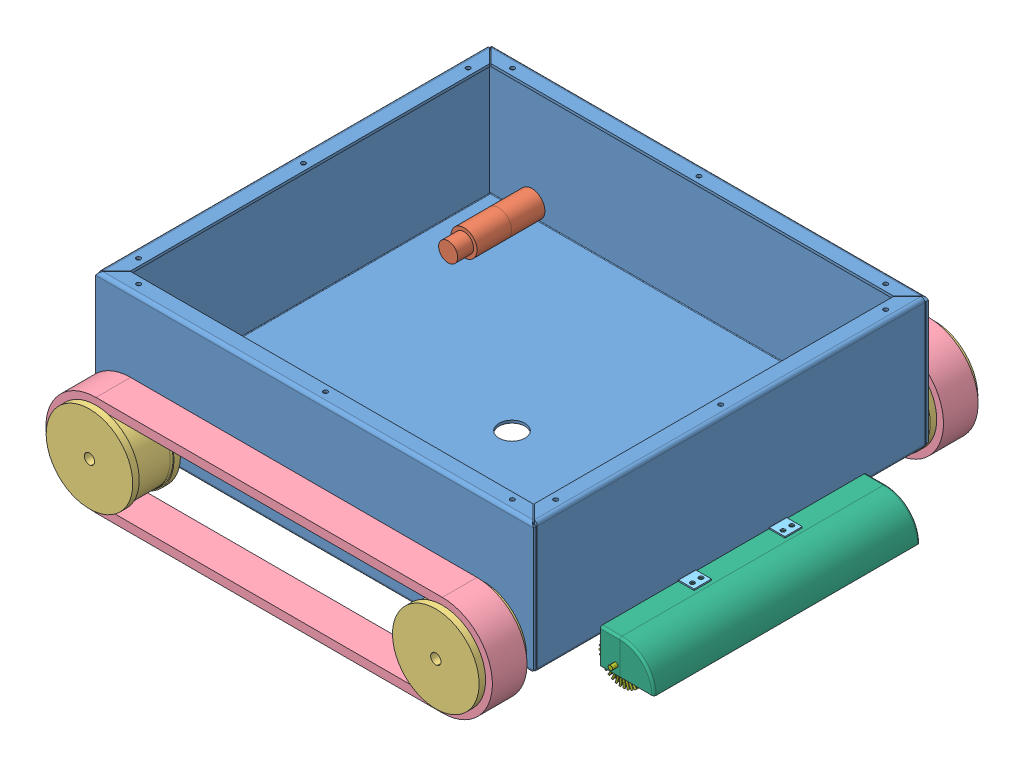
SolidWorks assembly Assem3, configuration Default. Lengths in mm.
Overall size (577.43 291.91 716.15).
15 component instances, 7 part files, 19 mates.
Components (placement in the parent):
- body-1: body [Default] at (194.2189 144.9067 418.1455) size (506.34 150.02 456.02)
- dunker-motor-2: dunker-motor [Default] at (-5.7811 160.6433 233.5455) x (0.813364 0.581754 0) z (0 0 -1) size (30 30 138.75)
- dunker-motor-3: dunker-motor [Default] at (394.2189 160.6433 233.5455) x (-0.923728 -0.383049 0) z (0 0 -1) size (30 30 138.75)
- dunker-motor-5: dunker-motor [Default] at (-5.7811 160.6433 602.7455) x (-0.974168 0.225824 0) z (0 0 1) size (30 30 138.75)
- dunker-motor-6: dunker-motor [Default] at (394.2189 160.6433 602.7455) x (-0.974168 0.225824 0) z (0 0 1) size (30 30 138.75)
- Rim1-1: Rim1 [Default] at (14.7798 166.9252 154.022) x (0 0 -1) z (0.292191 -0.95636 0) size (55 100 100)
- sair-1: sair [Default] at (120.0273 160.6433 177.6455) x (1 0 0) z (0 1 0) size (515.6 40 115.6)
- Rim1-2: Rim1 [Default] at (404.9847 179.2527 154.022) x (0 0 -1) z (0.86559 -0.500753 0) size (55 100 100)
- Rim1-3: Rim1 [Default] at (404.9847 179.2527 682.269) x (0 0 1) z (-0.86559 0.500753 0) size (55 100 100)
- sair-2: sair [Default] at (120.0273 160.6433 658.6455) x (1 0 0) z (0 -1 0) size (515.6 40 115.6)
- Rim1-4: Rim1 [Default] at (14.7798 166.9252 682.269) x (0 0 1) z (-0.292191 0.95636 0) size (55 100 100)
- cleaning part-1: cleaning part [Default] at (489.8925 -15.2578 313.6411) x (-1 0 0) z (0 1 0) size (115.57 320 56.98)
  - holder2-1: holder2 [Default] at (565.4382 75.7061 153.1645) size (72.07 200 12.5)
  - Part3-1: Part3 [Default] at (47.6736 218.1083 165.1645) x (-1 0 0) z (0 0 1) size (62 307 39.51)
  - brush 2-2: brush 2 [Default] at (24.6736 252.0044 137.1645) x (1 0 0) z (0 -1 0) size (52.04 51.98 320)
Mates (geometry in assembly coordinates):
- Concentric6: concentric aligned: cylinder of body-1 through (-5.7811 160.6433 190.138) axis (0 0 1) radius 3.25; cylinder of dunker-motor-2 through (-5.7811 160.6433 153.1455) axis (0 0 1) radius 3
- Coincident3: coincident anti-aligned: plane of body-1 through (194.2189 144.9067 193.1455) normal (0 0 1); plane of dunker-motor-2 through (-5.7811 160.6433 193.1455) normal (0 0 -1)
- Concentric7: concentric aligned: cylinder of body-1 through (394.2189 160.6433 190.138) axis (0 0 1) radius 3.25; cylinder of dunker-motor-3 through (394.2189 160.6433 153.1455) axis (0 0 1) radius 3
- Coincident4: coincident anti-aligned: plane of body-1 through (194.2189 144.9067 193.1455) normal (0 0 1); plane of dunker-motor-3 through (394.2189 160.6433 193.1455) normal (0 0 -1)
- Concentric9: concentric anti-aligned: line of body-1 through (-5.7811 160.6433 643.1455) axis (0 0 1); cylinder of dunker-motor-5 through (-5.7811 160.6433 683.1455) axis (0 0 -1) radius 3
- Coincident6: coincident anti-aligned: plane of body-1 through (194.2189 144.9067 643.1455) normal (0 0 -1); plane of dunker-motor-5 through (-5.7811 160.6433 643.1455) normal (0 0 1)
- Concentric10: concentric anti-aligned: cylinder of body-1 through (394.2189 160.6433 190.138) axis (0 0 1) radius 3.25; cylinder of dunker-motor-6 through (394.2189 160.6433 683.1455) axis (0 0 -1) radius 3
- Coincident7: coincident anti-aligned: plane of body-1 through (194.2189 144.9067 643.1455) normal (0 0 -1); plane of dunker-motor-6 through (394.2189 160.6433 643.1455) normal (0 0 1)
- Concentric11: concentric anti-aligned: cylinder of dunker-motor-2 through (-5.7811 160.6433 153.1455) axis (0 0 1) radius 3; cylinder of Rim1-1 through (-5.7811 160.6433 185.1455) axis (0 0 -1) radius 6
- Concentric12: concentric anti-aligned: cylinder of Rim1-1 through (-5.7811 160.6433 130.1455) axis (0 0 -1) radius 47.8; cylinder of sair-1 through (-5.7811 160.6433 137.6455) axis (0 0 1) radius 47.8
- Coincident8: coincident anti-aligned: plane of Rim1-1 through (42.0369 175.2529 177.6455) normal (0 0 -1); plane of sair-1 through (-5.7811 160.6433 177.6455) normal (0 0 1)
- Distance1: distance = 5 mm anti-aligned: plane of Rim1-1 through (34.1237 172.8352 185.1455) normal (0 0 1); plane of body-1 through (194.2189 144.9067 190.1455) normal (0 0 -1)
- Concentric13: concentric anti-aligned: cylinder of dunker-motor-3 through (394.2189 160.6433 153.1455) axis (0 0 1) radius 3; cylinder of Rim1-2 through (394.2189 160.6433 185.1455) axis (0 0 -1) radius 6
- Concentric14: concentric anti-aligned: cylinder of sair-1 through (394.2189 160.6433 137.6455) axis (0 0 1) radius 47.8; line of Rim1-2 through (394.2189 160.6433 203.6838) axis (0 0 -1)
- Coincident11: coincident anti-aligned: plane of sair-1 through (-5.7811 160.6433 177.6455) normal (0 0 1); plane of Rim1-2 through (419.2566 203.9228 177.6455) normal (0 0 -1)
- Parallel1: parallel anti-aligned: plane of body-1 through (447.2189 144.9067 418.1455) normal (1 0 0); plane of cleaning part-1/holder2-1 through (445.7189 137.9067 389.3472) normal (-1 0 0)
- Coincident15: coincident anti-aligned: plane of body-1 through (194.2189 141.9067 418.1455) normal (0 -1 0); plane of cleaning part-1/holder2-1 through (180.7043 141.9067 416.8724) normal (0 1 0)
- Coincident16: coincident anti-aligned: plane of body-1 through (447.2189 144.9067 418.1455) normal (1 0 0); plane of cleaning part-1/Part3-1 through (447.2189 149.9067 264.6455) normal (-1 0 0)
- Distance2: distance = 72 mm aligned: plane of cleaning part-1/Part3-1 through (447.2189 149.9067 262.1455) normal (0 0 -1); plane of body-1 through (194.2189 144.9067 190.1455) normal (0 0 -1)
